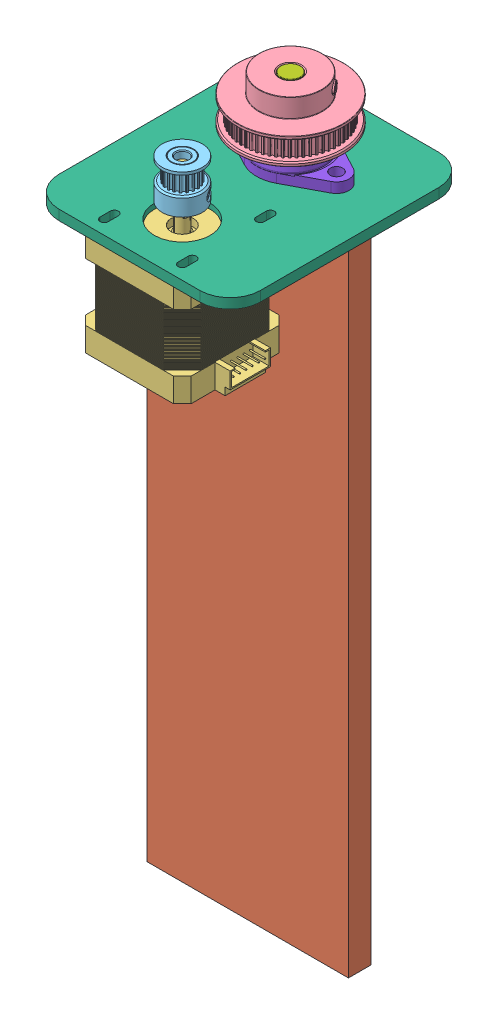
SolidWorks assembly Eje_Z, configuration Predeterminado. Lengths in mm.
Overall size (80 283.35 95).
15 component instances, 12 part files, 23 mates.
Components (placement in the parent):
- Eje_Z_guia_MGN12^Eje_Z-1: Eje_Z_guia_MGN12^Eje_Z [Predeterminado] at (56.2598 -105.1519 134.6514) x (1 0 0) z (0 1 0) size (9 6.61 250) (virtual)
- Copia de Placa_Motor^Eje_Z-1: Copia de Placa_Motor^Eje_Z [Predeterminado] at (70.7598 -105.1519 145.8457) x (-1 0 0) z (0 0 -1) size (80 250 9) (virtual)
-  Nema 17HS4401-S^Eje_Z-1:  Nema 17HS4401-S^Eje_Z [Varsayılan] at (30.7598 104.6481 171.8457) x (0 0 1) z (0 1 0) size (42 48 63.23) (virtual)
-  GT2_60T_8_6^Eje_Z-1:  GT2_60T_8_6^Eje_Z [Default] at (30.7598 170.6981 128.8457) x (0.816489 0 -0.577361) z (0 -1 0) size (42 42 18) (virtual)
- GT2_20T^Eje_Z-1: GT2_20T^Eje_Z [Конфигурация1] at (30.7598 154.7481 171.8457) x (0 1 0) z (-0.516573 0 -0.856243) size (16 16 16) (virtual)
- Copia de soporte_motor_Z^Eje_Z-1: Copia de soporte_motor_Z^Eje_Z [Predeterminado] at (-9.2402 148.8481 192.8457) x (0 0 -1) z (0 -1 0) size (95 80 4) (virtual)
- Copia de LeadScrew 8mm x 2mmPitch_eje_Z^Eje_Z-1: Copia de LeadScrew 8mm x 2mmPitch_eje_Z^Eje_Z [Default] at (30.7598 178.1981 128.8457) x (0.80721 0 -0.590265) z (0 1 0) size (8 8 283) (virtual)
- KFL08^Eje_Z-1: KFL08^Eje_Z [Varsayılan] at (30.7598 148.8481 128.8457) size (46.5 11.35 27) (virtual)
  - Copia de FLANGE^KFL08_Eje_Z-1: Copia de FLANGE^KFL08_Eje_Z [Default] at origin size (46.5 8.5 27) (virtual)
  - Copia de BEARING^KFL08_Eje_Z-1: Copia de BEARING^KFL08_Eje_Z [Default] at (0 4 0) x (1 0 0) z (0 -1 0) size (22 22 10.85) (virtual)
  - socket set screw cone point_am-1: socket set screw cone point_am [B18.3.6M - M2.5 x 0.45 x 2 Hex Socket Cone Pt. SS --S] at (0 9.425 5.45) x (0 0 -1) z (1 0 0) size (2 2.5 2.5)
  - socket set screw cone point_am-2: socket set screw cone point_am [B18.3.6M - M2.5 x 0.45 x 2 Hex Socket Cone Pt. SS --S] at (5.45 9.425 0) x (-1 0 0) z (0 0 -1) size (2 2.5 2.5)
- Eje_Z_guia_MGN12^Eje_Z-2: Eje_Z_guia_MGN12^Eje_Z [Predeterminado] at (5.2598 -105.1519 134.6514) x (1 0 0) z (0 1 0) size (9 6.61 250) (virtual)
- NEMA 23HS7430-1: NEMA 23HS7430 [По умолчанию] at (40.5598 155.7481 54.6457) x (1 0 0) z (0 -1 0) size (58.4 56.4 95.6) (hidden)
- Pieza1^Eje_Z-1: Pieza1^Eje_Z [Predeterminado] at origin (virtual)
Mates (geometry in assembly coordinates):
- Coincidente239: coincident anti-aligned: plane of Copia de Placa_Motor^Eje_Z-1 through (70.7598 144.8481 137.8457) normal (0 1 0); plane of Copia de soporte_motor_Z^Eje_Z-1 through (-9.2402 144.8481 192.8457) normal (0 -1 0)
- Coincidente240: coincident aligned: plane of Copia de Placa_Motor^Eje_Z-1 through (-9.2402 -105.1519 137.8457) normal (-1 0 0); plane of Copia de soporte_motor_Z^Eje_Z-1 through (-9.2402 144.8481 192.8457) normal (-1 0 0)
- Distancia1: distance = 47 mm aligned: plane of Copia de Placa_Motor^Eje_Z-1 through (70.7598 -105.1519 145.8457) normal (0 0 1); plane of Copia de soporte_motor_Z^Eje_Z-1 through (-9.2402 144.8481 192.8457) normal (0 0 1)
- Coincidente242: coincident anti-aligned: plane of  Nema 17HS4401-S^Eje_Z-1 through (30.7598 144.8481 171.8457) normal (0 1 0); plane of Copia de soporte_motor_Z^Eje_Z-1 through (-9.2402 144.8481 192.8457) normal (0 -1 0)
- Coincidente245: coincident anti-aligned: plane of Copia de soporte_motor_Z^Eje_Z-1 through (-9.2402 148.8481 192.8457) normal (0 1 0); plane of KFL08^Eje_Z-1/Copia de FLANGE^KFL08_Eje_Z-1 through (49.0098 148.8481 128.8457) normal (0 -1 0)
- Concéntrica10: concentric anti-aligned: cylinder of Copia de LeadScrew 8mm x 2mmPitch_eje_Z^Eje_Z-1 through (30.7598 -104.8019 128.8457) axis (0 1 0) radius 4; cylinder of KFL08^Eje_Z-1/Copia de BEARING^KFL08_Eje_Z-1 through (30.7598 149.3481 128.8457) axis (0 -1 0) radius 4
- Concéntrica11: concentric aligned: cylinder of  GT2_60T_8_6^Eje_Z-1 through (30.7598 140.6981 128.8457) axis (0 1 0) radius 4; cylinder of Copia de LeadScrew 8mm x 2mmPitch_eje_Z^Eje_Z-1 through (30.7598 -104.8019 128.8457) axis (0 1 0) radius 4
- Concéntrica12: concentric anti-aligned: cylinder of  Nema 17HS4401-S^Eje_Z-1 through (30.7598 167.8481 171.8457) axis (0 -1 0) radius 2.5; cylinder of GT2_20T^Eje_Z-1 through (30.7598 154.7481 171.8457) axis (0 1 0) radius 2.5
- Coincidente248: coincident aligned: plane of  GT2_60T_8_6^Eje_Z-1 through (30.7598 169.1981 128.8457) normal (0 -1 0); plane of GT2_20T^Eje_Z-1 through (30.7598 169.1981 171.8457) normal (0 -1 0)
- Coincidente249: coincident aligned: plane of  Nema 17HS4401-S^Eje_Z-1 through (13.2598 114.1481 192.8457) normal (0 0 1); plane of Copia de soporte_motor_Z^Eje_Z-1 through (-9.2402 144.8481 192.8457) normal (0 0 1)
- Distancia2: distance = 19 mm aligned: plane of  Nema 17HS4401-S^Eje_Z-1 through (9.7598 114.1481 154.3457) normal (-1 0 0); plane of Copia de soporte_motor_Z^Eje_Z-1 through (-9.2402 144.8481 192.8457) normal (-1 0 0)
- Coincidente250: coincident anti-aligned: plane of  GT2_60T_8_6^Eje_Z-1 through (30.7598 160.1981 128.8457) normal (0 -1 0); plane of KFL08^Eje_Z-1/Copia de BEARING^KFL08_Eje_Z-1 through (30.7598 160.1981 133.1457) normal (0 1 0)
- Concéntrica13: concentric aligned: cylinder of Copia de soporte_motor_Z^Eje_Z-1 through (30.7598 144.8481 128.8457) axis (0 1 0) radius 6; cylinder of Copia de LeadScrew 8mm x 2mmPitch_eje_Z^Eje_Z-1 through (30.7598 -104.8019 128.8457) axis (0 1 0) radius 4
- Coincidente252: coincident aligned: plane of  GT2_60T_8_6^Eje_Z-1 through (30.7598 178.1981 128.8457) normal (0 1 0); plane of Copia de LeadScrew 8mm x 2mmPitch_eje_Z^Eje_Z-1 through (30.7598 178.1981 128.8457) normal (0 1 0)
- Concéntrica14: concentric aligned: cylinder of Copia de soporte_motor_Z^Eje_Z-1 through (49.0098 144.8481 128.8457) axis (0 1 0) radius 1.625; cylinder of KFL08^Eje_Z-1/Copia de FLANGE^KFL08_Eje_Z-1 through (49.0098 152.8481 128.8457) axis (0 1 0) radius 2.5
- Coincidente253: coincident aligned: plane of NEMA 23HS7430-1 through (40.5598 157.3481 54.6457) normal (0 1 0); plane of KFL08^Eje_Z-1/Copia de FLANGE^KFL08_Eje_Z-1 through (18.0848 157.3481 128.8457) normal (0 1 0)
- Distancia3: distance = 2 mm aligned: plane of NEMA 23HS7430-1 through (68.7598 145.7481 26.4457) normal (1 0 0); plane of Copia de soporte_motor_Z^Eje_Z-1 through (70.7598 144.8481 192.8457) normal (1 0 0)
- Distancia4: distance = 55 mm anti-aligned: plane of Copia de Placa_Motor^Eje_Z-1 through (70.7598 -105.1519 137.8457) normal (0 0 -1); plane of NEMA 23HS7430-1 through (12.3598 145.7481 82.8457) normal (0 0 1)
- Coincidente254: coincident anti-aligned: plane of Eje_Z_guia_MGN12^Eje_Z-1 through (56.2598 -105.1519 137.8457) normal (0 0 1); plane of Copia de Placa_Motor^Eje_Z-1 through (70.7598 -105.1519 137.8457) normal (0 0 -1)
- Coincidente255: coincident anti-aligned: plane of Eje_Z_guia_MGN12^Eje_Z-1 through (60.7598 144.8481 137.8457) normal (1 0 0); plane of Copia de Placa_Motor^Eje_Z-1 through (60.7598 -105.1519 136.8457) normal (-1 0 0)
- Coincidente256: coincident aligned: plane of Eje_Z_guia_MGN12^Eje_Z-1 through (56.2598 -105.1519 134.6514) normal (0 -1 0); plane of Copia de Placa_Motor^Eje_Z-1 through (70.7598 -105.1519 137.8457) normal (0 -1 0)
- Coincidente257: coincident aligned: plane of Copia de Placa_Motor^Eje_Z-1 through (70.7598 -105.1519 137.8457) normal (0 -1 0); plane of Eje_Z_guia_MGN12^Eje_Z-2 through (5.2598 -105.1519 134.6514) normal (0 -1 0)
- Coincidente259: coincident anti-aligned: plane of Copia de Placa_Motor^Eje_Z-1 through (70.7598 -105.1519 137.8457) normal (0 0 -1); plane of Eje_Z_guia_MGN12^Eje_Z-2 through (5.2598 -105.1519 137.8457) normal (0 0 1)
